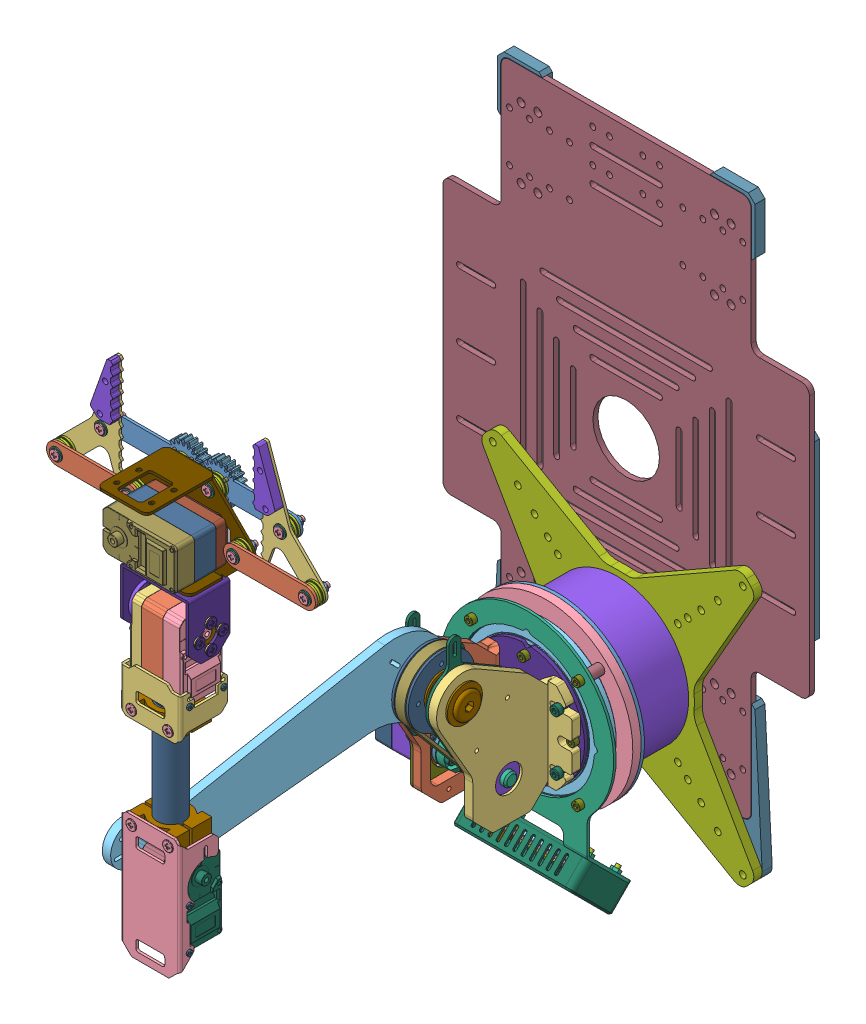
SolidWorks assembly RoArm-M1 STEP, configuration Default. Lengths in mm. (continued)
Components (placement in the parent): (continued)
- RoArm-M1 STEP(2)^RoArm-M1 STEP-1: RoArm-M1 STEP(2)^RoArm-M1 STEP [Default] at origin size (176.32 372.07 316.7) (virtual) (continued)
  - Servo Driver with ESP32^RoArm-M1 STEP(2)_RoArm-M1 STEP-1: Servo Driver with ESP32^RoArm-M1 STEP(2)_RoArm-M1 STEP [Default] at (-32.5 -89.0448 39.0323) x (1 0 0) z (0 -0.707107 0.707107) size (65.89 30.51 11.2) (virtual) (continued)
    - R14^Servo Driver with ESP32_RoArm-M1 STEP(2)_RoArm-M1 STEP-1: R14^Servo Driver with ESP32_RoArm-M1 STEP(2)_RoArm-M1 STEP [Default] at origin size (0.85 1.65 0.46) (virtual) (continued)
      - 490325008_10^R14_Servo Driver with ESP32_RoArm-M1 STEP(2)_RoArm-M1 STEP-1: 490325008_10^R14_Servo Driver with ESP32_RoArm-M1 STEP(2)_RoArm-M1 STEP [Default] at (17.7499 23.7937 -0.8715) size (0.85 0.28 0.46) (virtual)
        - Extruded (2)^490325008_10_R14_Servo Driver with ESP32_RoArm-M1 STEP(2)_RoArm-M1 STEP-1: Extruded (2)^490325008_10_R14_Servo Driver with ESP32_RoArm-M1 STEP(2)_RoArm-M1 STEP [Default] at origin size (0.85 0.28 0.46) (virtual)
      - 490325008_11^R14_Servo Driver with ESP32_RoArm-M1 STEP(2)_RoArm-M1 STEP-1: 490325008_11^R14_Servo Driver with ESP32_RoArm-M1 STEP(2)_RoArm-M1 STEP [Default] at (17.7499 22.4221 -0.8715) size (0.85 0.28 0.46) (virtual)
        - Extruded (2)^490325008_11_R14_Servo Driver with ESP32_RoArm-M1 STEP(2)_RoArm-M1 STEP-1: Extruded (2)^490325008_11_R14_Servo Driver with ESP32_RoArm-M1 STEP(2)_RoArm-M1 STEP [Default] at origin size (0.85 0.28 0.46) (virtual)
      - 490325136_5^R14_Servo Driver with ESP32_RoArm-M1 STEP(2)_RoArm-M1 STEP-1: 490325136_5^R14_Servo Driver with ESP32_RoArm-M1 STEP(2)_RoArm-M1 STEP [Default] at (17.7499 23.108 -0.8615) size (0.8 1.5 0.42) (virtual)
        - Extruded (3)^490325136_5_R14_Servo Driver with ESP32_RoArm-M1 STEP(2)_RoArm-M1 STEP-1: Extruded (3)^490325136_5_R14_Servo Driver with ESP32_RoArm-M1 STEP(2)_RoArm-M1 STEP [Default] at origin size (0.8 1.5 0.42) (virtual)
    - R12^Servo Driver with ESP32_RoArm-M1 STEP(2)_RoArm-M1 STEP-1: R12^Servo Driver with ESP32_RoArm-M1 STEP(2)_RoArm-M1 STEP [Default] at origin size (1.65 0.85 0.46) (virtual)
      - 490324624_32^R12_Servo Driver with ESP32_RoArm-M1 STEP(2)_RoArm-M1 STEP-1: 490324624_32^R12_Servo Driver with ESP32_RoArm-M1 STEP(2)_RoArm-M1 STEP [Default] at (20.8856 15.6078 -0.8715) size (0.28 0.85 0.46) (virtual)
        - Extruded (6)^490324624_32_R12_Servo Driver with ESP32_RoArm-M1 STEP(2)_RoArm-M1 STEP-1: Extruded (6)^490324624_32_R12_Servo Driver with ESP32_RoArm-M1 STEP(2)_RoArm-M1 STEP [Default] at origin size (0.28 0.85 0.46) (virtual)
      - 490324624_33^R12_Servo Driver with ESP32_RoArm-M1 STEP(2)_RoArm-M1 STEP-1: 490324624_33^R12_Servo Driver with ESP32_RoArm-M1 STEP(2)_RoArm-M1 STEP [Default] at (19.5141 15.6078 -0.8715) size (0.28 0.85 0.46) (virtual)
        - Extruded (6)^490324624_33_R12_Servo Driver with ESP32_RoArm-M1 STEP(2)_RoArm-M1 STEP-1: Extruded (6)^490324624_33_R12_Servo Driver with ESP32_RoArm-M1 STEP(2)_RoArm-M1 STEP [Default] at origin size (0.28 0.85 0.46) (virtual)
      - 490324752_16^R12_Servo Driver with ESP32_RoArm-M1 STEP(2)_RoArm-M1 STEP-1: 490324752_16^R12_Servo Driver with ESP32_RoArm-M1 STEP(2)_RoArm-M1 STEP [Default] at (20.1999 15.6078 -0.8615) size (1.5 0.8 0.42) (virtual)
        - Extruded (7)^490324752_16_R12_Servo Driver with ESP32_RoArm-M1 STEP(2)_RoArm-M1 STEP-1: Extruded (7)^490324752_16_R12_Servo Driver with ESP32_RoArm-M1 STEP(2)_RoArm-M1 STEP [Default] at origin size (1.5 0.8 0.42) (virtual)
    - R10^Servo Driver with ESP32_RoArm-M1 STEP(2)_RoArm-M1 STEP-1: R10^Servo Driver with ESP32_RoArm-M1 STEP(2)_RoArm-M1 STEP [Default] at origin size (1.65 0.85 0.46) (virtual)
      - 490324624_34^R10_Servo Driver with ESP32_RoArm-M1 STEP(2)_RoArm-M1 STEP-1: 490324624_34^R10_Servo Driver with ESP32_RoArm-M1 STEP(2)_RoArm-M1 STEP [Default] at (19.564 19.5079 -0.8715) size (0.28 0.85 0.46) (virtual)
        - Extruded (6)^490324624_34_R10_Servo Driver with ESP32_RoArm-M1 STEP(2)_RoArm-M1 STEP-1: Extruded (6)^490324624_34_R10_Servo Driver with ESP32_RoArm-M1 STEP(2)_RoArm-M1 STEP [Default] at origin size (0.28 0.85 0.46) (virtual)
      - 490324624_35^R10_Servo Driver with ESP32_RoArm-M1 STEP(2)_RoArm-M1 STEP-1: 490324624_35^R10_Servo Driver with ESP32_RoArm-M1 STEP(2)_RoArm-M1 STEP [Default] at (20.9355 19.5079 -0.8715) size (0.28 0.85 0.46) (virtual)
        - Extruded (6)^490324624_35_R10_Servo Driver with ESP32_RoArm-M1 STEP(2)_RoArm-M1 STEP-1: Extruded (6)^490324624_35_R10_Servo Driver with ESP32_RoArm-M1 STEP(2)_RoArm-M1 STEP [Default] at origin size (0.28 0.85 0.46) (virtual)
      - 490324752_17^R10_Servo Driver with ESP32_RoArm-M1 STEP(2)_RoArm-M1 STEP-1: 490324752_17^R10_Servo Driver with ESP32_RoArm-M1 STEP(2)_RoArm-M1 STEP [Default] at (20.2497 19.5079 -0.8615) size (1.5 0.8 0.42) (virtual)
        - Extruded (7)^490324752_17_R10_Servo Driver with ESP32_RoArm-M1 STEP(2)_RoArm-M1 STEP-1: Extruded (7)^490324752_17_R10_Servo Driver with ESP32_RoArm-M1 STEP(2)_RoArm-M1 STEP [Default] at origin size (1.5 0.8 0.42) (virtual)
    - R9^Servo Driver with ESP32_RoArm-M1 STEP(2)_RoArm-M1 STEP-1: R9^Servo Driver with ESP32_RoArm-M1 STEP(2)_RoArm-M1 STEP [Default] at origin size (1.65 0.85 0.46) (virtual)
      - 490324624_36^R9_Servo Driver with ESP32_RoArm-M1 STEP(2)_RoArm-M1 STEP-1: 490324624_36^R9_Servo Driver with ESP32_RoArm-M1 STEP(2)_RoArm-M1 STEP [Default] at (20.8856 17.1078 -0.8715) size (0.28 0.85 0.46) (virtual)
        - Extruded (6)^490324624_36_R9_Servo Driver with ESP32_RoArm-M1 STEP(2)_RoArm-M1 STEP-1: Extruded (6)^490324624_36_R9_Servo Driver with ESP32_RoArm-M1 STEP(2)_RoArm-M1 STEP [Default] at origin size (0.28 0.85 0.46) (virtual)
      - 490324624_37^R9_Servo Driver with ESP32_RoArm-M1 STEP(2)_RoArm-M1 STEP-1: 490324624_37^R9_Servo Driver with ESP32_RoArm-M1 STEP(2)_RoArm-M1 STEP [Default] at (19.5141 17.1078 -0.8715) size (0.28 0.85 0.46) (virtual)
        - Extruded (6)^490324624_37_R9_Servo Driver with ESP32_RoArm-M1 STEP(2)_RoArm-M1 STEP-1: Extruded (6)^490324624_37_R9_Servo Driver with ESP32_RoArm-M1 STEP(2)_RoArm-M1 STEP [Default] at origin size (0.28 0.85 0.46) (virtual)
      - 490324752_18^R9_Servo Driver with ESP32_RoArm-M1 STEP(2)_RoArm-M1 STEP-1: 490324752_18^R9_Servo Driver with ESP32_RoArm-M1 STEP(2)_RoArm-M1 STEP [Default] at (20.1999 17.1078 -0.8615) size (1.5 0.8 0.42) (virtual)
        - Extruded (7)^490324752_18_R9_Servo Driver with ESP32_RoArm-M1 STEP(2)_RoArm-M1 STEP-1: Extruded (7)^490324752_18_R9_Servo Driver with ESP32_RoArm-M1 STEP(2)_RoArm-M1 STEP [Default] at origin size (1.5 0.8 0.42) (virtual)
    - R8^Servo Driver with ESP32_RoArm-M1 STEP(2)_RoArm-M1 STEP-1: R8^Servo Driver with ESP32_RoArm-M1 STEP(2)_RoArm-M1 STEP [Default] at origin size (0.85 1.65 0.46) (virtual)
      - 490325008_12^R8_Servo Driver with ESP32_RoArm-M1 STEP(2)_RoArm-M1 STEP-1: 490325008_12^R8_Servo Driver with ESP32_RoArm-M1 STEP(2)_RoArm-M1 STEP [Default] at (13.4001 17.0858 -0.8715) size (0.85 0.28 0.46) (virtual)
        - Extruded (2)^490325008_12_R8_Servo Driver with ESP32_RoArm-M1 STEP(2)_RoArm-M1 STEP-1: Extruded (2)^490325008_12_R8_Servo Driver with ESP32_RoArm-M1 STEP(2)_RoArm-M1 STEP [Default] at origin size (0.85 0.28 0.46) (virtual)
      - 490325008_13^R8_Servo Driver with ESP32_RoArm-M1 STEP(2)_RoArm-M1 STEP-1: 490325008_13^R8_Servo Driver with ESP32_RoArm-M1 STEP(2)_RoArm-M1 STEP [Default] at (13.4001 15.7143 -0.8715) size (0.85 0.28 0.46) (virtual)
        - Extruded (2)^490325008_13_R8_Servo Driver with ESP32_RoArm-M1 STEP(2)_RoArm-M1 STEP-1: Extruded (2)^490325008_13_R8_Servo Driver with ESP32_RoArm-M1 STEP(2)_RoArm-M1 STEP [Default] at origin size (0.85 0.28 0.46) (virtual)
      - 490325136_6^R8_Servo Driver with ESP32_RoArm-M1 STEP(2)_RoArm-M1 STEP-1: 490325136_6^R8_Servo Driver with ESP32_RoArm-M1 STEP(2)_RoArm-M1 STEP [Default] at (13.4001 16.4001 -0.8615) size (0.8 1.5 0.42) (virtual)
        - Extruded (3)^490325136_6_R8_Servo Driver with ESP32_RoArm-M1 STEP(2)_RoArm-M1 STEP-1: Extruded (3)^490325136_6_R8_Servo Driver with ESP32_RoArm-M1 STEP(2)_RoArm-M1 STEP [Default] at origin size (0.8 1.5 0.42) (virtual)
    - R13^Servo Driver with ESP32_RoArm-M1 STEP(2)_RoArm-M1 STEP-1: R13^Servo Driver with ESP32_RoArm-M1 STEP(2)_RoArm-M1 STEP [Default] at origin size (1.65 0.85 0.46) (virtual)
      - 490324624_38^R13_Servo Driver with ESP32_RoArm-M1 STEP(2)_RoArm-M1 STEP-1: 490324624_38^R13_Servo Driver with ESP32_RoArm-M1 STEP(2)_RoArm-M1 STEP [Default] at (51.814 9.7078 0.001) size (0.28 0.85 0.46) (virtual)
        - Extruded (6)^490324624_38_R13_Servo Driver with ESP32_RoArm-M1 STEP(2)_RoArm-M1 STEP-1: Extruded (6)^490324624_38_R13_Servo Driver with ESP32_RoArm-M1 STEP(2)_RoArm-M1 STEP [Default] at origin size (0.28 0.85 0.46) (virtual)
      - 490324624_39^R13_Servo Driver with ESP32_RoArm-M1 STEP(2)_RoArm-M1 STEP-1: 490324624_39^R13_Servo Driver with ESP32_RoArm-M1 STEP(2)_RoArm-M1 STEP [Default] at (53.1855 9.7078 0.001) size (0.28 0.85 0.46) (virtual)
        - Extruded (6)^490324624_39_R13_Servo Driver with ESP32_RoArm-M1 STEP(2)_RoArm-M1 STEP-1: Extruded (6)^490324624_39_R13_Servo Driver with ESP32_RoArm-M1 STEP(2)_RoArm-M1 STEP [Default] at origin size (0.28 0.85 0.46) (virtual)
      - 490324752_19^R13_Servo Driver with ESP32_RoArm-M1 STEP(2)_RoArm-M1 STEP-1: 490324752_19^R13_Servo Driver with ESP32_RoArm-M1 STEP(2)_RoArm-M1 STEP [Default] at (52.4997 9.7078 0.025) size (1.5 0.8 0.42) (virtual)
        - Extruded (7)^490324752_19_R13_Servo Driver with ESP32_RoArm-M1 STEP(2)_RoArm-M1 STEP-1: Extruded (7)^490324752_19_R13_Servo Driver with ESP32_RoArm-M1 STEP(2)_RoArm-M1 STEP [Default] at origin size (1.5 0.8 0.42) (virtual)
    - R11^Servo Driver with ESP32_RoArm-M1 STEP(2)_RoArm-M1 STEP-1: R11^Servo Driver with ESP32_RoArm-M1 STEP(2)_RoArm-M1 STEP [Default] at origin size (1.65 0.85 0.46) (virtual)
      - 490324624_40^R11_Servo Driver with ESP32_RoArm-M1 STEP(2)_RoArm-M1 STEP-1: 490324624_40^R11_Servo Driver with ESP32_RoArm-M1 STEP(2)_RoArm-M1 STEP [Default] at (54.7674 9.7078 0.001) size (0.28 0.85 0.46) (virtual)
        - Extruded (6)^490324624_40_R11_Servo Driver with ESP32_RoArm-M1 STEP(2)_RoArm-M1 STEP-1: Extruded (6)^490324624_40_R11_Servo Driver with ESP32_RoArm-M1 STEP(2)_RoArm-M1 STEP [Default] at origin size (0.28 0.85 0.46) (virtual)
      - 490324624_41^R11_Servo Driver with ESP32_RoArm-M1 STEP(2)_RoArm-M1 STEP-1: 490324624_41^R11_Servo Driver with ESP32_RoArm-M1 STEP(2)_RoArm-M1 STEP [Default] at (56.1389 9.7078 0.001) size (0.28 0.85 0.46) (virtual)
        - Extruded (6)^490324624_41_R11_Servo Driver with ESP32_RoArm-M1 STEP(2)_RoArm-M1 STEP-1: Extruded (6)^490324624_41_R11_Servo Driver with ESP32_RoArm-M1 STEP(2)_RoArm-M1 STEP [Default] at origin size (0.28 0.85 0.46) (virtual)
      - 490324752_20^R11_Servo Driver with ESP32_RoArm-M1 STEP(2)_RoArm-M1 STEP-1: 490324752_20^R11_Servo Driver with ESP32_RoArm-M1 STEP(2)_RoArm-M1 STEP [Default] at (55.4531 9.7078 0.025) size (1.5 0.8 0.42) (virtual)
        - Extruded (7)^490324752_20_R11_Servo Driver with ESP32_RoArm-M1 STEP(2)_RoArm-M1 STEP-1: Extruded (7)^490324752_20_R11_Servo Driver with ESP32_RoArm-M1 STEP(2)_RoArm-M1 STEP [Default] at origin size (1.5 0.8 0.42) (virtual)
    - R7^Servo Driver with ESP32_RoArm-M1 STEP(2)_RoArm-M1 STEP-1: R7^Servo Driver with ESP32_RoArm-M1 STEP(2)_RoArm-M1 STEP [Default] at origin size (0.85 1.65 0.46) (virtual)
      - 490325008_14^R7_Servo Driver with ESP32_RoArm-M1 STEP(2)_RoArm-M1 STEP-1: 490325008_14^R7_Servo Driver with ESP32_RoArm-M1 STEP(2)_RoArm-M1 STEP [Default] at (56.8501 21.8358 -0.8715) size (0.85 0.28 0.46) (virtual)
        - Extruded (2)^490325008_14_R7_Servo Driver with ESP32_RoArm-M1 STEP(2)_RoArm-M1 STEP-1: Extruded (2)^490325008_14_R7_Servo Driver with ESP32_RoArm-M1 STEP(2)_RoArm-M1 STEP [Default] at origin size (0.85 0.28 0.46) (virtual)
      - 490325008_15^R7_Servo Driver with ESP32_RoArm-M1 STEP(2)_RoArm-M1 STEP-1: 490325008_15^R7_Servo Driver with ESP32_RoArm-M1 STEP(2)_RoArm-M1 STEP [Default] at (56.8501 20.4643 -0.8715) size (0.85 0.28 0.46) (virtual)
        - Extruded (2)^490325008_15_R7_Servo Driver with ESP32_RoArm-M1 STEP(2)_RoArm-M1 STEP-1: Extruded (2)^490325008_15_R7_Servo Driver with ESP32_RoArm-M1 STEP(2)_RoArm-M1 STEP [Default] at origin size (0.85 0.28 0.46) (virtual)
      - 490325136_7^R7_Servo Driver with ESP32_RoArm-M1 STEP(2)_RoArm-M1 STEP-1: 490325136_7^R7_Servo Driver with ESP32_RoArm-M1 STEP(2)_RoArm-M1 STEP [Default] at (56.8501 21.1501 -0.8615) size (0.8 1.5 0.42) (virtual)
        - Extruded (3)^490325136_7_R7_Servo Driver with ESP32_RoArm-M1 STEP(2)_RoArm-M1 STEP-1: Extruded (3)^490325136_7_R7_Servo Driver with ESP32_RoArm-M1 STEP(2)_RoArm-M1 STEP [Default] at origin size (0.8 1.5 0.42) (virtual)
    - R6^Servo Driver with ESP32_RoArm-M1 STEP(2)_RoArm-M1 STEP-1: R6^Servo Driver with ESP32_RoArm-M1 STEP(2)_RoArm-M1 STEP [Default] at origin size (0.85 1.65 0.46) (virtual)
      - 490325008_16^R6_Servo Driver with ESP32_RoArm-M1 STEP(2)_RoArm-M1 STEP-1: 490325008_16^R6_Servo Driver with ESP32_RoArm-M1 STEP(2)_RoArm-M1 STEP [Default] at (25.6499 9.172 0.001) size (0.85 0.28 0.46) (virtual)
        - Extruded (2)^490325008_16_R6_Servo Driver with ESP32_RoArm-M1 STEP(2)_RoArm-M1 STEP-1: Extruded (2)^490325008_16_R6_Servo Driver with ESP32_RoArm-M1 STEP(2)_RoArm-M1 STEP [Default] at origin size (0.85 0.28 0.46) (virtual)
      - 490325008_17^R6_Servo Driver with ESP32_RoArm-M1 STEP(2)_RoArm-M1 STEP-1: 490325008_17^R6_Servo Driver with ESP32_RoArm-M1 STEP(2)_RoArm-M1 STEP [Default] at (25.6499 10.5436 0.001) size (0.85 0.28 0.46) (virtual)
        - Extruded (2)^490325008_17_R6_Servo Driver with ESP32_RoArm-M1 STEP(2)_RoArm-M1 STEP-1: Extruded (2)^490325008_17_R6_Servo Driver with ESP32_RoArm-M1 STEP(2)_RoArm-M1 STEP [Default] at origin size (0.85 0.28 0.46) (virtual)
      - 490325136_8^R6_Servo Driver with ESP32_RoArm-M1 STEP(2)_RoArm-M1 STEP-1: 490325136_8^R6_Servo Driver with ESP32_RoArm-M1 STEP(2)_RoArm-M1 STEP [Default] at (25.6499 9.8578 0.025) size (0.8 1.5 0.42) (virtual)
        - Extruded (3)^490325136_8_R6_Servo Driver with ESP32_RoArm-M1 STEP(2)_RoArm-M1 STEP-1: Extruded (3)^490325136_8_R6_Servo Driver with ESP32_RoArm-M1 STEP(2)_RoArm-M1 STEP [Default] at origin size (0.8 1.5 0.42) (virtual)
    - Q1^Servo Driver with ESP32_RoArm-M1 STEP(2)_RoArm-M1 STEP-1: Q1^Servo Driver with ESP32_RoArm-M1 STEP(2)_RoArm-M1 STEP [Default] at origin size (2.9 3.58 0.55) (virtual)
      - 490331664^Q1_Servo Driver with ESP32_RoArm-M1 STEP(2)_RoArm-M1 STEP-1: 490331664^Q1_Servo Driver with ESP32_RoArm-M1 STEP(2)_RoArm-M1 STEP [Default] at (20.2473 23.6201 -0.5715) size (0.58 1.17 0.16) (virtual)
        - Extruded (15)^490331664_Q1_Servo Driver with ESP32_RoArm-M1 STEP(2)_RoArm-M1 STEP-1: Extruded (15)^490331664_Q1_Servo Driver with ESP32_RoArm-M1 STEP(2)_RoArm-M1 STEP [Default] at origin size (0.58 1.17 0.16) (virtual)
      - 490331024^Q1_Servo Driver with ESP32_RoArm-M1 STEP(2)_RoArm-M1 STEP-1: 490331024^Q1_Servo Driver with ESP32_RoArm-M1 STEP(2)_RoArm-M1 STEP [Default] at (20.2498 22.4079 -0.9615) size (2.9 1.3 0.5) (virtual)
        - Extruded (16)^490331024_Q1_Servo Driver with ESP32_RoArm-M1 STEP(2)_RoArm-M1 STEP-1: Extruded (16)^490331024_Q1_Servo Driver with ESP32_RoArm-M1 STEP(2)_RoArm-M1 STEP [Default] at origin size (2.9 1.3 0.5) (virtual)
      - 490331664_1^Q1_Servo Driver with ESP32_RoArm-M1 STEP(2)_RoArm-M1 STEP-1: 490331664_1^Q1_Servo Driver with ESP32_RoArm-M1 STEP(2)_RoArm-M1 STEP [Default] at (21.2125 21.2071 -0.5715) size (0.58 1.17 0.16) (virtual)
        - Extruded (15)^490331664_1_Q1_Servo Driver with ESP32_RoArm-M1 STEP(2)_RoArm-M1 STEP-1: Extruded (15)^490331664_1_Q1_Servo Driver with ESP32_RoArm-M1 STEP(2)_RoArm-M1 STEP [Default] at origin size (0.58 1.17 0.16) (virtual)
      - 490331664_2^Q1_Servo Driver with ESP32_RoArm-M1 STEP(2)_RoArm-M1 STEP-1: 490331664_2^Q1_Servo Driver with ESP32_RoArm-M1 STEP(2)_RoArm-M1 STEP [Default] at (19.2821 21.2071 -0.5715) size (0.58 1.17 0.16) (virtual)
        - Extruded (15)^490331664_2_Q1_Servo Driver with ESP32_RoArm-M1 STEP(2)_RoArm-M1 STEP-1: Extruded (15)^490331664_2_Q1_Servo Driver with ESP32_RoArm-M1 STEP(2)_RoArm-M1 STEP [Default] at origin size (0.58 1.17 0.16) (virtual)
    - PWR4^Servo Driver with ESP32_RoArm-M1 STEP(2)_RoArm-M1 STEP-1: PWR4^Servo Driver with ESP32_RoArm-M1 STEP(2)_RoArm-M1 STEP [Default] at origin size (0.85 1.65 0.46) (virtual)
      - 490325008_18^PWR4_Servo Driver with ESP32_RoArm-M1 STEP(2)_RoArm-M1 STEP-1: 490325008_18^PWR4_Servo Driver with ESP32_RoArm-M1 STEP(2)_RoArm-M1 STEP [Default] at (45.4501 9.672 -0.8715) size (0.85 0.28 0.46) (virtual)
        - Extruded (2)^490325008_18_PWR4_Servo Driver with ESP32_RoArm-M1 STEP(2)_RoArm-M1 STEP-1: Extruded (2)^490325008_18_PWR4_Servo Driver with ESP32_RoArm-M1 STEP(2)_RoArm-M1 STEP [Default] at origin size (0.85 0.28 0.46) (virtual)
      - 490325008_19^PWR4_Servo Driver with ESP32_RoArm-M1 STEP(2)_RoArm-M1 STEP-1: 490325008_19^PWR4_Servo Driver with ESP32_RoArm-M1 STEP(2)_RoArm-M1 STEP [Default] at (45.4501 11.0436 -0.8715) size (0.85 0.28 0.46) (virtual)
        - Extruded (2)^490325008_19_PWR4_Servo Driver with ESP32_RoArm-M1 STEP(2)_RoArm-M1 STEP-1: Extruded (2)^490325008_19_PWR4_Servo Driver with ESP32_RoArm-M1 STEP(2)_RoArm-M1 STEP [Default] at origin size (0.85 0.28 0.46) (virtual)
      - 490325136_9^PWR4_Servo Driver with ESP32_RoArm-M1 STEP(2)_RoArm-M1 STEP-1: 490325136_9^PWR4_Servo Driver with ESP32_RoArm-M1 STEP(2)_RoArm-M1 STEP [Default] at (45.4501 10.3578 -0.8615) size (0.8 1.5 0.42) (virtual)
        - Extruded (3)^490325136_9_PWR4_Servo Driver with ESP32_RoArm-M1 STEP(2)_RoArm-M1 STEP-1: Extruded (3)^490325136_9_PWR4_Servo Driver with ESP32_RoArm-M1 STEP(2)_RoArm-M1 STEP [Default] at origin size (0.8 1.5 0.42) (virtual)
    - PWR3^Servo Driver with ESP32_RoArm-M1 STEP(2)_RoArm-M1 STEP-1: PWR3^Servo Driver with ESP32_RoArm-M1 STEP(2)_RoArm-M1 STEP [Default] at origin size (1.51 3.44 0.46) (virtual)
      - 490328720_2^PWR3_Servo Driver with ESP32_RoArm-M1 STEP(2)_RoArm-M1 STEP-1: 490328720_2^PWR3_Servo Driver with ESP32_RoArm-M1 STEP(2)_RoArm-M1 STEP [Default] at (47.3003 8.7079 -0.8715) size (1.51 0.28 0.46) (virtual)
        - Extruded^490328720_2_PWR3_Servo Driver with ESP32_RoArm-M1 STEP(2)_RoArm-M1 STEP-1: Extruded^490328720_2_PWR3_Servo Driver with ESP32_RoArm-M1 STEP(2)_RoArm-M1 STEP [Default] at origin size (1.51 0.28 0.46) (virtual)
      - 490328720_3^PWR3_Servo Driver with ESP32_RoArm-M1 STEP(2)_RoArm-M1 STEP-1: 490328720_3^PWR3_Servo Driver with ESP32_RoArm-M1 STEP(2)_RoArm-M1 STEP [Default] at (47.3002 11.8703 -0.8715) size (1.51 0.28 0.46) (virtual)
        - Extruded^490328720_3_PWR3_Servo Driver with ESP32_RoArm-M1 STEP(2)_RoArm-M1 STEP-1: Extruded^490328720_3_PWR3_Servo Driver with ESP32_RoArm-M1 STEP(2)_RoArm-M1 STEP [Default] at origin size (1.51 0.28 0.46) (virtual)
      - 731907408_1^PWR3_Servo Driver with ESP32_RoArm-M1 STEP(2)_RoArm-M1 STEP-1: 731907408_1^PWR3_Servo Driver with ESP32_RoArm-M1 STEP(2)_RoArm-M1 STEP [Default] at (47.2923 10.2829 -0.8615) size (1.38 3.05 0.42) (virtual)
        - Extruded (1)^731907408_1_PWR3_Servo Driver with ESP32_RoArm-M1 STEP(2)_RoArm-M1 STEP-1: Extruded (1)^731907408_1_PWR3_Servo Driver with ESP32_RoArm-M1 STEP(2)_RoArm-M1 STEP [Default] at origin size (1.38 3.05 0.42) (virtual)
    - PWR2^Servo Driver with ESP32_RoArm-M1 STEP(2)_RoArm-M1 STEP-1: PWR2^Servo Driver with ESP32_RoArm-M1 STEP(2)_RoArm-M1 STEP [Default] at origin size (0.85 1.65 0.46) (virtual)
      - 490325008_20^PWR2_Servo Driver with ESP32_RoArm-M1 STEP(2)_RoArm-M1 STEP-1: 490325008_20^PWR2_Servo Driver with ESP32_RoArm-M1 STEP(2)_RoArm-M1 STEP [Default] at (23.2001 2.3142 0.001) size (0.85 0.28 0.46) (virtual)
        - Extruded (2)^490325008_20_PWR2_Servo Driver with ESP32_RoArm-M1 STEP(2)_RoArm-M1 STEP-1: Extruded (2)^490325008_20_PWR2_Servo Driver with ESP32_RoArm-M1 STEP(2)_RoArm-M1 STEP [Default] at origin size (0.85 0.28 0.46) (virtual)
      - 490325008_21^PWR2_Servo Driver with ESP32_RoArm-M1 STEP(2)_RoArm-M1 STEP-1: 490325008_21^PWR2_Servo Driver with ESP32_RoArm-M1 STEP(2)_RoArm-M1 STEP [Default] at (23.2001 3.6857 0.001) size (0.85 0.28 0.46) (virtual)
        - Extruded (2)^490325008_21_PWR2_Servo Driver with ESP32_RoArm-M1 STEP(2)_RoArm-M1 STEP-1: Extruded (2)^490325008_21_PWR2_Servo Driver with ESP32_RoArm-M1 STEP(2)_RoArm-M1 STEP [Default] at origin size (0.85 0.28 0.46) (virtual)
      - 490325136_10^PWR2_Servo Driver with ESP32_RoArm-M1 STEP(2)_RoArm-M1 STEP-1: 490325136_10^PWR2_Servo Driver with ESP32_RoArm-M1 STEP(2)_RoArm-M1 STEP [Default] at (23.2001 2.9999 0.025) size (0.8 1.5 0.42) (virtual)
        - Extruded (3)^490325136_10_PWR2_Servo Driver with ESP32_RoArm-M1 STEP(2)_RoArm-M1 STEP-1: Extruded (3)^490325136_10_PWR2_Servo Driver with ESP32_RoArm-M1 STEP(2)_RoArm-M1 STEP [Default] at origin size (0.8 1.5 0.42) (virtual)
    - PWR1^Servo Driver with ESP32_RoArm-M1 STEP(2)_RoArm-M1 STEP-1: PWR1^Servo Driver with ESP32_RoArm-M1 STEP(2)_RoArm-M1 STEP [Default] at origin size (3.44 1.51 0.46) (virtual)
      - 490328208^PWR1_Servo Driver with ESP32_RoArm-M1 STEP(2)_RoArm-M1 STEP-1: 490328208^PWR1_Servo Driver with ESP32_RoArm-M1 STEP(2)_RoArm-M1 STEP [Default] at (56.8001 9.1499 -0.8715) size (0.28 1.51 0.46) (virtual)
        - Extruded (17)^490328208_PWR1_Servo Driver with ESP32_RoArm-M1 STEP(2)_RoArm-M1 STEP-1: Extruded (17)^490328208_PWR1_Servo Driver with ESP32_RoArm-M1 STEP(2)_RoArm-M1 STEP [Default] at origin size (0.28 1.51 0.46) (virtual)
      - 490328208_1^PWR1_Servo Driver with ESP32_RoArm-M1 STEP(2)_RoArm-M1 STEP-1: 490328208_1^PWR1_Servo Driver with ESP32_RoArm-M1 STEP(2)_RoArm-M1 STEP [Default] at (59.9625 9.15 -0.8715) size (0.28 1.51 0.46) (virtual)
        - Extruded (17)^490328208_1_PWR1_Servo Driver with ESP32_RoArm-M1 STEP(2)_RoArm-M1 STEP-1: Extruded (17)^490328208_1_PWR1_Servo Driver with ESP32_RoArm-M1 STEP(2)_RoArm-M1 STEP [Default] at origin size (0.28 1.51 0.46) (virtual)
      - 513869488^PWR1_Servo Driver with ESP32_RoArm-M1 STEP(2)_RoArm-M1 STEP-1: 513869488^PWR1_Servo Driver with ESP32_RoArm-M1 STEP(2)_RoArm-M1 STEP [Default] at (58.375 9.1579 -0.8615) size (3.05 1.38 0.42) (virtual)
        - Extruded (18)^513869488_PWR1_Servo Driver with ESP32_RoArm-M1 STEP(2)_RoArm-M1 STEP-1: Extruded (18)^513869488_PWR1_Servo Driver with ESP32_RoArm-M1 STEP(2)_RoArm-M1 STEP [Default] at origin size (3.05 1.38 0.42) (virtual)
    - D1^Servo Driver with ESP32_RoArm-M1 STEP(2)_RoArm-M1 STEP-1: D1^Servo Driver with ESP32_RoArm-M1 STEP(2)_RoArm-M1 STEP [Default] at origin size (4.1 1.84 1.3) (virtual)
      - 490329488^D1_Servo Driver with ESP32_RoArm-M1 STEP(2)_RoArm-M1 STEP-1: 490329488^D1_Servo Driver with ESP32_RoArm-M1 STEP(2)_RoArm-M1 STEP [Default] at (19.3999 1.1878 -1.9115) size (4.1 1.84 1.3) (virtual)
        - Extruded (19)^490329488_D1_Servo Driver with ESP32_RoArm-M1 STEP(2)_RoArm-M1 STEP-1: Extruded (19)^490329488_D1_Servo Driver with ESP32_RoArm-M1 STEP(2)_RoArm-M1 STEP [Default] at origin size (4.1 1.84 1.3) (virtual)
    - AMS-1^Servo Driver with ESP32_RoArm-M1 STEP(2)_RoArm-M1 STEP-1: AMS-1^Servo Driver with ESP32_RoArm-M1 STEP(2)_RoArm-M1 STEP [Default] at origin size (6.73 3.43 1.02) (virtual)
      - 490330512^AMS-1_Servo Driver with ESP32_RoArm-M1 STEP(2)_RoArm-M1 STEP-1: 490330512^AMS-1_Servo Driver with ESP32_RoArm-M1 STEP(2)_RoArm-M1 STEP [Default] at (52.1373 9.7901 -1.6815) size (6.73 3.43 1.02) (virtual)
        - Extruded (20)^490330512_AMS-1_Servo Driver with ESP32_RoArm-M1 STEP(2)_RoArm-M1 STEP-1: Extruded (20)^490330512_AMS-1_Servo Driver with ESP32_RoArm-M1 STEP(2)_RoArm-M1 STEP [Default] at origin size (6.73 3.43 1.02) (virtual)
    - M1^Servo Driver with ESP32_RoArm-M1 STEP(2)_RoArm-M1 STEP-1: M1^Servo Driver with ESP32_RoArm-M1 STEP(2)_RoArm-M1 STEP [Default] at origin size (17.65 25.15 2.3) (virtual)
      - 731906256^M1_Servo Driver with ESP32_RoArm-M1 STEP(2)_RoArm-M1 STEP-1: 731906256^M1_Servo Driver with ESP32_RoArm-M1 STEP(2)_RoArm-M1 STEP [Default] at (32.8248 17.3329 -0.8615) size (17.65 25.15 0.42) (virtual)
        - Extruded (21)^731906256_M1_Servo Driver with ESP32_RoArm-M1 STEP(2)_RoArm-M1 STEP-1: Extruded (21)^731906256_M1_Servo Driver with ESP32_RoArm-M1 STEP(2)_RoArm-M1 STEP [Default] at origin size (17.65 25.15 0.42) (virtual)
      - 731905872^M1_Servo Driver with ESP32_RoArm-M1 STEP(2)_RoArm-M1 STEP-1: 731905872^M1_Servo Driver with ESP32_RoArm-M1 STEP(2)_RoArm-M1 STEP [Default] at (32.8498 14.6579 -2.7115) size (16.3 18.6 2.3) (virtual)
        - Extruded (22)^731905872_M1_Servo Driver with ESP32_RoArm-M1 STEP(2)_RoArm-M1 STEP-1: Extruded (22)^731905872_M1_Servo Driver with ESP32_RoArm-M1 STEP(2)_RoArm-M1 STEP [Default] at origin size (16.3 18.6 2.3) (virtual)
    - C1^Servo Driver with ESP32_RoArm-M1 STEP(2)_RoArm-M1 STEP-1: C1^Servo Driver with ESP32_RoArm-M1 STEP(2)_RoArm-M1 STEP [Default] at origin size (0.85 1.65 0.46) (virtual)
      - 490325136_11^C1_Servo Driver with ESP32_RoArm-M1 STEP(2)_RoArm-M1 STEP-1: 490325136_11^C1_Servo Driver with ESP32_RoArm-M1 STEP(2)_RoArm-M1 STEP [Default] at (56.8497 15.0112 -0.8615) size (0.8 1.5 0.42) (virtual)
        - Extruded (3)^490325136_11_C1_Servo Driver with ESP32_RoArm-M1 STEP(2)_RoArm-M1 STEP-1: Extruded (3)^490325136_11_C1_Servo Driver with ESP32_RoArm-M1 STEP(2)_RoArm-M1 STEP [Default] at origin size (0.8 1.5 0.42) (virtual)
      - 490325008_22^C1_Servo Driver with ESP32_RoArm-M1 STEP(2)_RoArm-M1 STEP-1: 490325008_22^C1_Servo Driver with ESP32_RoArm-M1 STEP(2)_RoArm-M1 STEP [Default] at (56.8497 15.697 -0.8715) size (0.85 0.28 0.46) (virtual)
        - Extruded (2)^490325008_22_C1_Servo Driver with ESP32_RoArm-M1 STEP(2)_RoArm-M1 STEP-1: Extruded (2)^490325008_22_C1_Servo Driver with ESP32_RoArm-M1 STEP(2)_RoArm-M1 STEP [Default] at origin size (0.85 0.28 0.46) (virtual)
      - 490325008_23^C1_Servo Driver with ESP32_RoArm-M1 STEP(2)_RoArm-M1 STEP-1: 490325008_23^C1_Servo Driver with ESP32_RoArm-M1 STEP(2)_RoArm-M1 STEP [Default] at (56.8497 14.3254 -0.8715) size (0.85 0.28 0.46) (virtual)
        - Extruded (2)^490325008_23_C1_Servo Driver with ESP32_RoArm-M1 STEP(2)_RoArm-M1 STEP-1: Extruded (2)^490325008_23_C1_Servo Driver with ESP32_RoArm-M1 STEP(2)_RoArm-M1 STEP [Default] at origin size (0.85 0.28 0.46) (virtual)
    - C2^Servo Driver with ESP32_RoArm-M1 STEP(2)_RoArm-M1 STEP-1: C2^Servo Driver with ESP32_RoArm-M1 STEP(2)_RoArm-M1 STEP [Default] at origin size (1.65 0.85 0.46) (virtual)
      - 490324752_21^C2_Servo Driver with ESP32_RoArm-M1 STEP(2)_RoArm-M1 STEP-1: 490324752_21^C2_Servo Driver with ESP32_RoArm-M1 STEP(2)_RoArm-M1 STEP [Default] at (43.5497 8.6578 0.025) size (1.5 0.8 0.42) (virtual)
        - Extruded (7)^490324752_21_C2_Servo Driver with ESP32_RoArm-M1 STEP(2)_RoArm-M1 STEP-1: Extruded (7)^490324752_21_C2_Servo Driver with ESP32_RoArm-M1 STEP(2)_RoArm-M1 STEP [Default] at origin size (1.5 0.8 0.42) (virtual)
      - 490324624_42^C2_Servo Driver with ESP32_RoArm-M1 STEP(2)_RoArm-M1 STEP-1: 490324624_42^C2_Servo Driver with ESP32_RoArm-M1 STEP(2)_RoArm-M1 STEP [Default] at (44.2355 8.6578 0.001) size (0.28 0.85 0.46) (virtual)
        - Extruded (6)^490324624_42_C2_Servo Driver with ESP32_RoArm-M1 STEP(2)_RoArm-M1 STEP-1: Extruded (6)^490324624_42_C2_Servo Driver with ESP32_RoArm-M1 STEP(2)_RoArm-M1 STEP [Default] at origin size (0.28 0.85 0.46) (virtual)
      - 490324624_43^C2_Servo Driver with ESP32_RoArm-M1 STEP(2)_RoArm-M1 STEP-1: 490324624_43^C2_Servo Driver with ESP32_RoArm-M1 STEP(2)_RoArm-M1 STEP [Default] at (42.864 8.6578 0.001) size (0.28 0.85 0.46) (virtual)
        - Extruded (6)^490324624_43_C2_Servo Driver with ESP32_RoArm-M1 STEP(2)_RoArm-M1 STEP-1: Extruded (6)^490324624_43_C2_Servo Driver with ESP32_RoArm-M1 STEP(2)_RoArm-M1 STEP [Default] at origin size (0.28 0.85 0.46) (virtual)
    - C3^Servo Driver with ESP32_RoArm-M1 STEP(2)_RoArm-M1 STEP-1: C3^Servo Driver with ESP32_RoArm-M1 STEP(2)_RoArm-M1 STEP [Default] at origin size (1.65 0.85 0.46) (virtual)
      - 490324752_22^C3_Servo Driver with ESP32_RoArm-M1 STEP(2)_RoArm-M1 STEP-1: 490324752_22^C3_Servo Driver with ESP32_RoArm-M1 STEP(2)_RoArm-M1 STEP [Default] at (43.5497 10.1578 0.025) size (1.5 0.8 0.42) (virtual)
        - Extruded (7)^490324752_22_C3_Servo Driver with ESP32_RoArm-M1 STEP(2)_RoArm-M1 STEP-1: Extruded (7)^490324752_22_C3_Servo Driver with ESP32_RoArm-M1 STEP(2)_RoArm-M1 STEP [Default] at origin size (1.5 0.8 0.42) (virtual)
      - 490324624_44^C3_Servo Driver with ESP32_RoArm-M1 STEP(2)_RoArm-M1 STEP-1: 490324624_44^C3_Servo Driver with ESP32_RoArm-M1 STEP(2)_RoArm-M1 STEP [Default] at (44.2355 10.1578 0.001) size (0.28 0.85 0.46) (virtual)
        - Extruded (6)^490324624_44_C3_Servo Driver with ESP32_RoArm-M1 STEP(2)_RoArm-M1 STEP-1: Extruded (6)^490324624_44_C3_Servo Driver with ESP32_RoArm-M1 STEP(2)_RoArm-M1 STEP [Default] at origin size (0.28 0.85 0.46) (virtual)
      - 490324624_45^C3_Servo Driver with ESP32_RoArm-M1 STEP(2)_RoArm-M1 STEP-1: 490324624_45^C3_Servo Driver with ESP32_RoArm-M1 STEP(2)_RoArm-M1 STEP [Default] at (42.864 10.1578 0.001) size (0.28 0.85 0.46) (virtual)
        - Extruded (6)^490324624_45_C3_Servo Driver with ESP32_RoArm-M1 STEP(2)_RoArm-M1 STEP-1: Extruded (6)^490324624_45_C3_Servo Driver with ESP32_RoArm-M1 STEP(2)_RoArm-M1 STEP [Default] at origin size (0.28 0.85 0.46) (virtual)
    - C4^Servo Driver with ESP32_RoArm-M1 STEP(2)_RoArm-M1 STEP-1: C4^Servo Driver with ESP32_RoArm-M1 STEP(2)_RoArm-M1 STEP [Default] at origin size (1.65 0.85 0.46) (virtual)
      - 490324752_23^C4_Servo Driver with ESP32_RoArm-M1 STEP(2)_RoArm-M1 STEP-1: 490324752_23^C4_Servo Driver with ESP32_RoArm-M1 STEP(2)_RoArm-M1 STEP [Default] at (14.2001 18.7001 0.025) size (1.5 0.8 0.42) (virtual)
        - Extruded (7)^490324752_23_C4_Servo Driver with ESP32_RoArm-M1 STEP(2)_RoArm-M1 STEP-1: Extruded (7)^490324752_23_C4_Servo Driver with ESP32_RoArm-M1 STEP(2)_RoArm-M1 STEP [Default] at origin size (1.5 0.8 0.42) (virtual)
      - 490324624_46^C4_Servo Driver with ESP32_RoArm-M1 STEP(2)_RoArm-M1 STEP-1: 490324624_46^C4_Servo Driver with ESP32_RoArm-M1 STEP(2)_RoArm-M1 STEP [Default] at (13.5143 18.7001 0.001) size (0.28 0.85 0.46) (virtual)
        - Extruded (6)^490324624_46_C4_Servo Driver with ESP32_RoArm-M1 STEP(2)_RoArm-M1 STEP-1: Extruded (6)^490324624_46_C4_Servo Driver with ESP32_RoArm-M1 STEP(2)_RoArm-M1 STEP [Default] at origin size (0.28 0.85 0.46) (virtual)
      - 490324624_47^C4_Servo Driver with ESP32_RoArm-M1 STEP(2)_RoArm-M1 STEP-1: 490324624_47^C4_Servo Driver with ESP32_RoArm-M1 STEP(2)_RoArm-M1 STEP [Default] at (14.8858 18.7001 0.001) size (0.28 0.85 0.46) (virtual)
        - Extruded (6)^490324624_47_C4_Servo Driver with ESP32_RoArm-M1 STEP(2)_RoArm-M1 STEP-1: Extruded (6)^490324624_47_C4_Servo Driver with ESP32_RoArm-M1 STEP(2)_RoArm-M1 STEP [Default] at origin size (0.28 0.85 0.46) (virtual)
    - C5^Servo Driver with ESP32_RoArm-M1 STEP(2)_RoArm-M1 STEP-1: C5^Servo Driver with ESP32_RoArm-M1 STEP(2)_RoArm-M1 STEP [Default] at origin size (1.65 0.85 0.46) (virtual)
      - 490324752_24^C5_Servo Driver with ESP32_RoArm-M1 STEP(2)_RoArm-M1 STEP-1: 490324752_24^C5_Servo Driver with ESP32_RoArm-M1 STEP(2)_RoArm-M1 STEP [Default] at (14.5997 23.8579 -0.8615) size (1.5 0.8 0.42) (virtual)
        - Extruded (7)^490324752_24_C5_Servo Driver with ESP32_RoArm-M1 STEP(2)_RoArm-M1 STEP-1: Extruded (7)^490324752_24_C5_Servo Driver with ESP32_RoArm-M1 STEP(2)_RoArm-M1 STEP [Default] at origin size (1.5 0.8 0.42) (virtual)
      - 490324624_48^C5_Servo Driver with ESP32_RoArm-M1 STEP(2)_RoArm-M1 STEP-1: 490324624_48^C5_Servo Driver with ESP32_RoArm-M1 STEP(2)_RoArm-M1 STEP [Default] at (15.2855 23.8579 -0.8715) size (0.28 0.85 0.46) (virtual)
        - Extruded (6)^490324624_48_C5_Servo Driver with ESP32_RoArm-M1 STEP(2)_RoArm-M1 STEP-1: Extruded (6)^490324624_48_C5_Servo Driver with ESP32_RoArm-M1 STEP(2)_RoArm-M1 STEP [Default] at origin size (0.28 0.85 0.46) (virtual)
      - 490324624_49^C5_Servo Driver with ESP32_RoArm-M1 STEP(2)_RoArm-M1 STEP-1: 490324624_49^C5_Servo Driver with ESP32_RoArm-M1 STEP(2)_RoArm-M1 STEP [Default] at (13.914 23.8579 -0.8715) size (0.28 0.85 0.46) (virtual)
        - Extruded (6)^490324624_49_C5_Servo Driver with ESP32_RoArm-M1 STEP(2)_RoArm-M1 STEP-1: Extruded (6)^490324624_49_C5_Servo Driver with ESP32_RoArm-M1 STEP(2)_RoArm-M1 STEP [Default] at origin size (0.28 0.85 0.46) (virtual)
    - C6^Servo Driver with ESP32_RoArm-M1 STEP(2)_RoArm-M1 STEP-1: C6^Servo Driver with ESP32_RoArm-M1 STEP(2)_RoArm-M1 STEP [Default] at origin size (1.65 0.85 0.46) (virtual)
      - 490324752_25^C6_Servo Driver with ESP32_RoArm-M1 STEP(2)_RoArm-M1 STEP-1: 490324752_25^C6_Servo Driver with ESP32_RoArm-M1 STEP(2)_RoArm-M1 STEP [Default] at (49.4497 9.7078 0.025) size (1.5 0.8 0.42) (virtual)
        - Extruded (7)^490324752_25_C6_Servo Driver with ESP32_RoArm-M1 STEP(2)_RoArm-M1 STEP-1: Extruded (7)^490324752_25_C6_Servo Driver with ESP32_RoArm-M1 STEP(2)_RoArm-M1 STEP [Default] at origin size (1.5 0.8 0.42) (virtual)
      - 490324624_50^C6_Servo Driver with ESP32_RoArm-M1 STEP(2)_RoArm-M1 STEP-1: 490324624_50^C6_Servo Driver with ESP32_RoArm-M1 STEP(2)_RoArm-M1 STEP [Default] at (50.1355 9.7078 0.001) size (0.28 0.85 0.46) (virtual)
        - Extruded (6)^490324624_50_C6_Servo Driver with ESP32_RoArm-M1 STEP(2)_RoArm-M1 STEP-1: Extruded (6)^490324624_50_C6_Servo Driver with ESP32_RoArm-M1 STEP(2)_RoArm-M1 STEP [Default] at origin size (0.28 0.85 0.46) (virtual)
      - 490324624_51^C6_Servo Driver with ESP32_RoArm-M1 STEP(2)_RoArm-M1 STEP-1: 490324624_51^C6_Servo Driver with ESP32_RoArm-M1 STEP(2)_RoArm-M1 STEP [Default] at (48.764 9.7078 0.001) size (0.28 0.85 0.46) (virtual)
        - Extruded (6)^490324624_51_C6_Servo Driver with ESP32_RoArm-M1 STEP(2)_RoArm-M1 STEP-1: Extruded (6)^490324624_51_C6_Servo Driver with ESP32_RoArm-M1 STEP(2)_RoArm-M1 STEP [Default] at origin size (0.28 0.85 0.46) (virtual)
    - C12^Servo Driver with ESP32_RoArm-M1 STEP(2)_RoArm-M1 STEP-1: C12^Servo Driver with ESP32_RoArm-M1 STEP(2)_RoArm-M1 STEP [Default] at origin size (0.85 1.65 0.46) (virtual)
      - 490325136_12^C12_Servo Driver with ESP32_RoArm-M1 STEP(2)_RoArm-M1 STEP-1: 490325136_12^C12_Servo Driver with ESP32_RoArm-M1 STEP(2)_RoArm-M1 STEP [Default] at (45.7759 20.5757 -0.8615) size (0.8 1.5 0.42) (virtual)
        - Extruded (3)^490325136_12_C12_Servo Driver with ESP32_RoArm-M1 STEP(2)_RoArm-M1 STEP-1: Extruded (3)^490325136_12_C12_Servo Driver with ESP32_RoArm-M1 STEP(2)_RoArm-M1 STEP [Default] at origin size (0.8 1.5 0.42) (virtual)
      - 490325008_24^C12_Servo Driver with ESP32_RoArm-M1 STEP(2)_RoArm-M1 STEP-1: 490325008_24^C12_Servo Driver with ESP32_RoArm-M1 STEP(2)_RoArm-M1 STEP [Default] at (45.7759 19.8899 -0.8715) size (0.85 0.28 0.46) (virtual)
